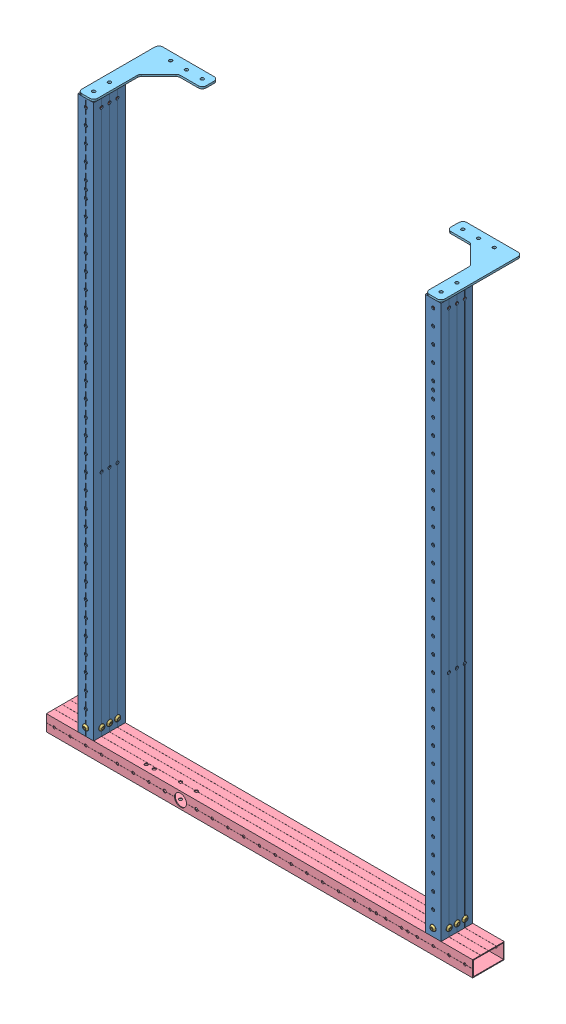
SolidWorks assembly 1 Stage, configuration Default. Lengths in mm.
Overall size (685.8 917.58 129.57).
11 component instances, 5 part files, 18 mates.
Components (placement in the parent):
- 1 Stage Vertical Versaframe-3: 1 Stage Vertical Versaframe [Default] at (317.3981 -180.3729 2090.2896) size (25.4 889 50.8)
- Block-1: Block [Default] at (-1067.0924 -53.3729 2090.0991) x (0 -1 0) z (0 0 1) size (20.64 21.84 47.24)
- Block screws-1: Block screws [Default] at (-12.8019 -180.3729 2090.2896) size (30.55 21.45 55.95)
- 1 Stage Vertical Versaframe-4: 1 Stage Vertical Versaframe [Default] at (545.9981 -180.3729 2090.2896) x (-1 0 0) z (0 0 -1) size (25.4 889 50.8)
- Block-2: Block [Default] at (1930.4886 -53.3729 2090.0991) x (0 -1 0) z (0 0 -1) size (20.64 21.84 47.24)
- Block screws-3: Block screws [Default] at (545.9981 -180.3729 2090.2896) size (30.55 21.45 55.95)
- Crossbar-1: Crossbar [Default] at (25.2981 -180.3729 2090.2896) x (0 1 0) z (-1 0 0) size (25.4 50.8 685.8)
- Block-3: Block [Default] at (-1066.9019 607.0271 2090.2896) x (0 1 0) z (0 0 -1) size (20.64 21.84 47.24)
- Block-4: Block [Default] at (-508.1019 607.0271 2090.2896) x (0 1 0) z (0 0 -1) size (20.64 21.84 47.24)
- Pulley Mount Bracket-1: Pulley Mount Bracket [Default] at (164.9981 721.3271 2115.6896) x (-1 0 0) z (0 0 -1) size (86.36 3.17 127)
- Pulley Mount Bracket-2: Pulley Mount Bracket [Default] at (698.3981 724.5021 2115.6896) x (1 0 0) z (0 0 -1) size (86.36 3.17 127)
Mates (geometry in assembly coordinates):
- Coincident13: coincident aligned: plane of 1 Stage Vertical Versaframe-3 through (152.2981 -167.6729 2090.2896) normal (0 -1 0); plane of Block-1 through (152.1076 -167.6729 2090.0991) normal (0 -1 0)
- Coincident14: coincident anti-aligned: plane of 1 Stage Vertical Versaframe-3 through (141.1856 -167.6729 2090.2896) normal (1 0 0); plane of Block-1 through (141.1856 -148.6229 2113.7211) normal (-1 0 0)
- Coincident15: coincident anti-aligned: plane of 1 Stage Vertical Versaframe-3 through (152.2981 -167.6729 2066.4771) normal (0 0 1); plane of Block-1 through (141.1856 -148.6229 2066.4771) normal (0 0 -1)
- Concentric7: concentric aligned: circle of 1 Stage Vertical Versaframe-3; circle of Block screws-1
- Coincident16: coincident anti-aligned: plane of 1 Stage Vertical Versaframe-3 through (139.5981 -167.6729 2115.6896) normal (-1 0 0); plane of Block screws-1 through (139.5981 -154.9729 2077.5896) normal (1 0 0)
- Coincident17: coincident anti-aligned: plane of 1 Stage Vertical Versaframe-3 through (164.9981 -167.6729 2064.8896) normal (0 0 -1); plane of Block screws-1 through (152.2981 -154.9729 2064.8896) normal (0 0 1)
- Concentric16: concentric aligned: cylinder of 1 Stage Vertical Versaframe-4 through (723.7981 -154.9729 2102.9896) axis (-1 0 0) radius 2.4892; cylinder of Block screws-3 through (707.9231 -154.9729 2102.9896) axis (-1 0 0) radius 2.3749
- Coincident27: coincident anti-aligned: plane of 1 Stage Vertical Versaframe-4 through (698.3981 -167.6729 2064.8896) normal (-1 0 0); plane of Block screws-3 through (698.3981 -154.9729 2102.9896) normal (1 0 0)
- Parallel7: parallel anti-aligned: plane of 1 Stage Vertical Versaframe-4 through (698.3981 -167.6729 2064.8896) normal (0 0 -1); plane of Block screws-3 through (711.0981 -154.9729 2064.8896) normal (0 0 1)
- Coincident30: coincident anti-aligned: plane of 1 Stage Vertical Versaframe-4 through (711.0981 -167.6729 2090.2896) normal (0 -1 0); plane of Crossbar-1 through (-724.0019 -167.6729 2115.6896) normal (0 1 0)
- Coincident31: coincident aligned: plane of 1 Stage Vertical Versaframe-4 through (698.3981 -167.6729 2064.8896) normal (0 0 -1); plane of Crossbar-1 through (-724.0019 -193.0729 2064.8896) normal (0 0 -1)
- Distance2: distance = 50.8 mm aligned: plane of Crossbar-1 through (774.5981 -180.3729 2090.2896) normal (1 0 0); plane of 1 Stage Vertical Versaframe-4 through (723.7981 -167.6729 2064.8896) normal (1 0 0)
- Concentric25: concentric aligned: circle of 1 Stage Vertical Versaframe-3; circle of Block-3
- Concentric26: concentric anti-aligned: circle of 1 Stage Vertical Versaframe-3; circle of Block-3
- Width1: width aligned: plane of Block-3 through (141.3761 702.2771 2066.6676) normal (-1 0 0); plane of 1 Stage Vertical Versaframe-3 through (163.2201 702.2771 2066.6676) normal (1 0 0); plane of Block-3 through (163.4106 -167.6729 2090.2896) normal (-1 0 0); plane of 1 Stage Vertical Versaframe-3 through (141.1856 -167.6729 2090.2896) normal (1 0 0)
- Coincident44: coincident anti-aligned: plane of Block-3 through (152.2981 721.3271 2090.2896) normal (0 1 0); plane of Pulley Mount Bracket-1 through (164.9981 721.3271 2115.6896) normal (0 -1 0)
- Concentric29: concentric anti-aligned: circle of Block-3; cylinder of Pulley Mount Bracket-1 through (152.2981 724.5021 2102.9896) axis (0 -1 0) radius 2.54
- Concentric30: concentric aligned: circle of Block-3; circle of Pulley Mount Bracket-1
